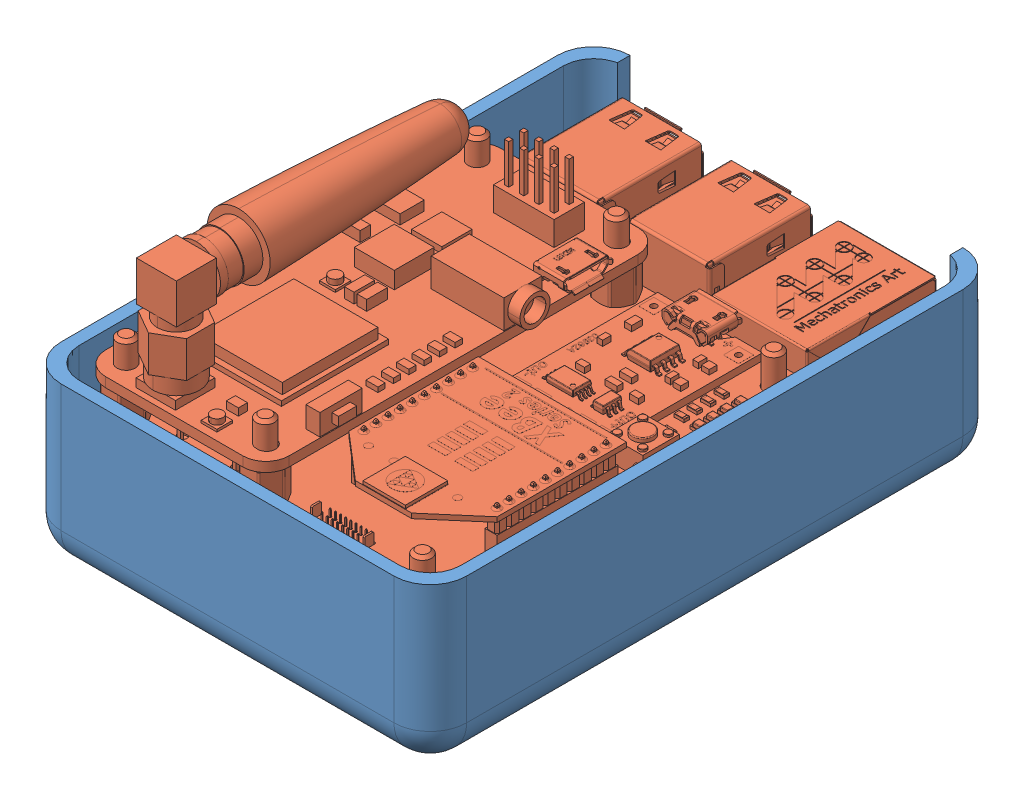
SolidWorks assembly Box&OBD, configuration По умолчанию. Lengths in mm.
Overall size (69.44 48.52 94).
2 component instances, 2 part files, 1 mates.
Components (placement in the parent):
- Box_SmartOBD-1: Box_SmartOBD [По умолчанию] at (14.7265 35.9676 110.6537) size (67 27 94)
- Smart_OBD-1: Smart_OBD [По умолчанию] at (-143.612 53.8061 17.5643) x (1 0 0) z (0 -1 0) size (66.98 89.87 48.52)
Mates (geometry in assembly coordinates):
- Совпадение1: coincident anti-aligned: plane of Box_SmartOBD-1 through (14.7265 40.9676 110.6537) normal (0 1 0); plane of Smart_OBD-1 through (67.7623 40.9676 29.8521) normal (0 -1 0)
